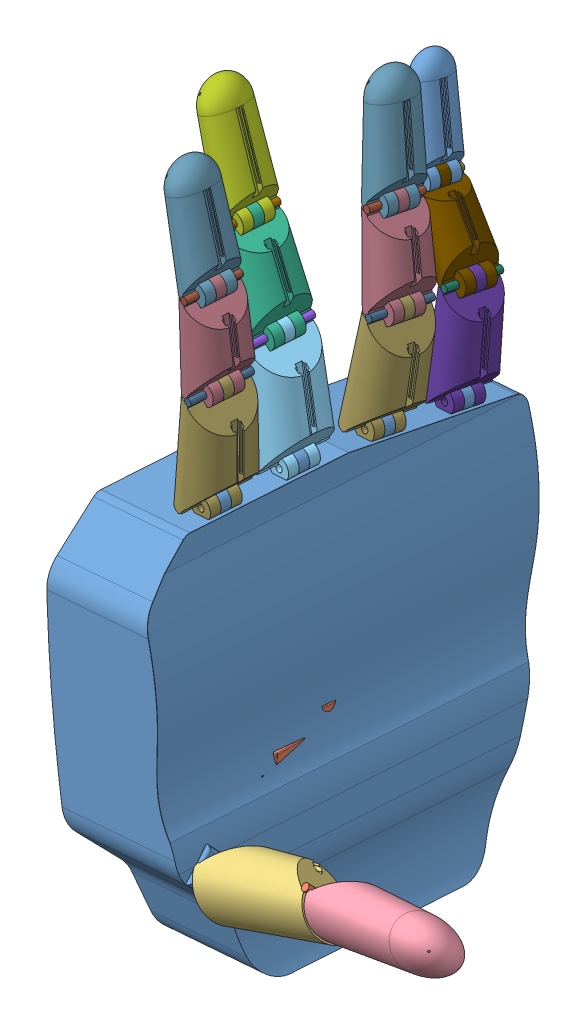
SolidWorks assembly hand_ass, configuration Default. Lengths in mm.
Overall size (398.4 729.74 146.06).
29 component instances, 20 part files, 46 mates.
Components (placement in the parent):
- mainbody_v2-4: mainbody_v2 [Default] at (1134.5845 69.0185 158.0505) x (0.046641 -0.018599 -0.998739) z (0.99192 0.118954 0.044107) size (116.82 635.31 320.58)
- Mate1t-4: Mate1t [Default] at (1191.8966 45.3831 191.6287) x (-0.116407 0.715114 0.689247) z (0.676171 0.565369 -0.472388) size (23 2 2)
- Part1t-3: Part1t [Default] at (1176.7391 49.6304 201.3469) x (-0.116407 0.715114 0.689247) z (-0.223805 0.65723 -0.719694) size (25.41 37 18.49)
- Part2t-3: Part2t [Default] at (1207.7668 55.7981 200.1909) x (-0.116407 0.715114 0.689247) z (-0.080418 0.6849 -0.724186) size (22.13 38.57 15.06)
- Part1m-2: Part1m [Default] at (1137.6384 140.5256 161.7486) x (0.046641 -0.018599 -0.998739) z (0.98582 0.162199 0.043017) size (21.28 37 15.36)
- Part2m-2: Part2m [Default] at (1130.0953 167.3581 160.8968) x (0.046641 -0.018599 -0.998739) z (0.920688 0.388657 0.035758) size (18.99 32 13.25)
- Part3m-2: Part3m [Default] at (1120.5618 193.9579 159.9559) x (0.046641 -0.018599 -0.998739) z (0.948492 0.31446 0.038438) size (16.1 35.5 11.04)
- Mate1-2: Mate1 [Default] at (1135.4417 155.2011 170.3841) x (0.046641 -0.018599 -0.998739) z (0.869405 0.4931 0.031418) size (18 2 2)
- Mate2-2: Mate2 [Default] at (1125.4133 179.1336 168.469) x (0.046641 -0.018599 -0.998739) z (0.879503 0.4748 0.032231) size (16 2 2)
- Mate1i-7: Mate1i [Default] at (1143.3187 152.4098 142.8187) x (0.061583 -0.147495 -0.987144) z (0.853826 0.519985 -0.024429) size (18 2 2)
- Mate2i-7: Mate2i [Default] at (1138.9313 172.9705 122.2515) x (-0.061583 0.147495 0.987144) z (-0.994862 0.070561 -0.072607) size (16 2 2)
- Part1i-6: Part1i [Default] at (1142.4486 137.6017 135.8591) x (0.061583 -0.147495 -0.987144) z (0.996376 -0.04906 0.069489) size (21.16 35 15.37)
- Part2-6: Part2 [Default] at (1140.4752 163.0002 131.9417) x (0.061583 -0.147495 -0.987144) z (0.972078 0.233235 0.025794) size (18.98 30 13.22)
- Part3i-6: Part3i [Default] at (1135.3592 188.4508 127.8194) x (0.061583 -0.147495 -0.987144) z (0.979901 0.196947 0.031704) size (16.1 33.51 11.04)
- Mate1p-2: Mate1p [Default] at (1142.4314 147.9759 119.6197) x (0.061583 -0.147495 -0.987144) z (0.991698 -0.102811 0.077228) size (16 2 2)
- Mate2p-2: Mate2p [Default] at (1128.4407 165.688 115.0872) x (0.061583 -0.147495 -0.987144) z (0.997523 0.042777 0.055839) size (14 2 2)
- Part1p-2: Part1p [Default] at (1142.7215 133.6027 113.6812) x (0.061583 -0.147495 -0.987144) z (0.997846 0.031496 0.057544) size (18.99 34 13.27)
- Part2p-2: Part2p [Default] at (1135.3313 155.7282 109.9141) x (0.061583 -0.147495 -0.987144) z (0.789257 0.612605 -0.042295) size (16.86 29 11.21)
- Part3p-2: Part3p [Default] at (1125.6893 177.679 106.0327) x (0.061583 -0.147495 -0.987144) z (0.9741 0.224473 0.027229) size (14.11 31.5 9.04)
- Mate1i-8: Mate1i [Default] at (1140.5368 153.6877 174.7899) x (-0.046641 0.018599 0.998739) z (-0.986648 -0.157045 -0.043151) size (18 2 2)
- Mate2i-8: Mate2i [Default] at (1137.6969 177.5363 175.215) x (-0.046641 0.018599 0.998739) z (-0.918896 -0.39289 -0.035595) size (16 2 2)
- Part1i-7: Part1i [Default] at (1139.3564 140.1863 183.9975) x (0.046641 -0.018599 -0.998739) z (0.998861 -0.009171 0.046817) size (21.16 35 15.37)
- Part2-7: Part2 [Default] at (1138.0875 166.2375 183.4538) x (0.046641 -0.018599 -0.998739) z (0.992108 0.117354 0.044146) size (18.98 30 13.22)
- Part3i-7: Part3i [Default] at (1133.0697 191.866 182.7419) x (0.046641 -0.018599 -0.998739) z (0.961902 0.270471 0.039884) size (16.1 33.51 11.04)
- SERVO 2-2: SERVO 2 [Default] at (1148.3811 12.1609 137.2372) x (0.109846 0.09566 0.989335) z (-0.993739 0.031034 0.107334) size (32 28.96 12.1)
- SERVO 2-3: SERVO 2 [Default] at (1148.2867 43.8698 121.8028) x (0.181431 0.08615 0.979623) z (-0.982404 -0.029015 0.184498) size (32 28.96 12.1)
- SERVO 2-4: SERVO 2 [Default] at (1157.2242 73.2498 119.0491) x (-0.09534 0.112725 0.989042) z (-0.991573 0.076792 -0.104336) size (32 28.96 12.1)
- SERVO 2-6: SERVO 2 [Default] at (1161.1471 38.2643 160.3978) x (0.061151 0.042032 0.997243) z (-0.997289 0.043545 0.059319) size (32 28.96 12.1)
- SERVO 2-7: SERVO 2 [Default] at (1116.2743 78.6077 176.2963) x (0.262447 -0.043955 -0.963945) z (0.96317 -0.048661 0.264455) size (32 28.96 12.1)
Mates (geometry in assembly coordinates):
- Concentric1: concentric anti-aligned: cylinder of mainbody_v2-4 through (1139.8961 124.8334 182.8072) axis (-0.046641 0.018599 0.998739) radius 1; cylinder of Part1i-7 through (1139.3299 125.0592 194.9299) axis (0.046641 -0.018599 -0.998739) radius 1
- Coincident1: coincident anti-aligned: plane of mainbody_v2-4 through (1139.8961 124.8334 182.8072) normal (0.046641 -0.018599 -0.998739); plane of Part1i-7 through (1139.8961 124.8334 182.8072) normal (-0.046641 0.018599 0.998739)
- Concentric2: concentric aligned: cylinder of Part1i-7 through (1139.6208 154.0529 194.4036) axis (0.046641 -0.018599 -0.998739) radius 1; cylinder of Part2-7 through (1139.6736 154.0319 193.2733) axis (0.046641 -0.018599 -0.998739) radius 1
- Coincident2: coincident anti-aligned: plane of Part1i-7 through (1140.047 153.883 185.277) normal (-0.046641 0.018599 0.998739); plane of Part2-7 through (1140.047 153.883 185.277) normal (0.046641 -0.018599 -0.998739)
- Concentric3: concentric aligned: cylinder of Mate1i-8 through (1139.6972 154.0225 192.7672) axis (0.046641 -0.018599 -0.998739) radius 1; cylinder of Part2-7 through (1139.6736 154.0319 193.2733) axis (0.046641 -0.018599 -0.998739) radius 1
- Coincident3: coincident anti-aligned: plane of Mate1i-8 through (1140.117 153.8551 183.7785) normal (-0.046641 0.018599 0.998739); plane of Part1i-7 through (1139.3564 140.1863 183.9975) normal (0.046641 -0.018599 -0.998739)
- Concentric4: concentric anti-aligned: cylinder of Part2-7 through (1136.8804 177.8619 192.6991) axis (0.046641 -0.018599 -0.998739) radius 1; cylinder of Part3i-7 through (1137.6736 177.5456 175.7142) axis (-0.046641 0.018599 0.998739) radius 1
- Coincident4: coincident anti-aligned: plane of Part2-7 through (1137.3937 177.6572 181.7066) normal (0.046641 -0.018599 -0.998739); plane of Part3i-7 through (1137.3937 177.6572 181.7066) normal (-0.046641 0.018599 0.998739)
- Concentric5: concentric anti-aligned: cylinder of Mate2i-8 through (1136.9506 177.8339 191.1948) axis (0.046641 -0.018599 -0.998739) radius 1; cylinder of Part3i-7 through (1137.6736 177.5456 175.7142) axis (-0.046641 0.018599 0.998739) radius 1
- Coincident5: coincident anti-aligned: plane of Mate2i-8 through (1137.3237 177.6851 183.2049) normal (-0.046641 0.018599 0.998739); plane of Part2-7 through (1138.0875 166.2375 183.4538) normal (0.046641 -0.018599 -0.998739)
- Concentric6: concentric anti-aligned: cylinder of mainbody_v2-4 through (1140.9285 124.4218 160.7001) axis (-0.046641 0.018599 0.998739) radius 1; cylinder of Part1m-2 through (1140.3622 124.6476 172.8256) axis (0.046641 -0.018599 -0.998739) radius 1
- Coincident6: coincident anti-aligned: plane of mainbody_v2-4 through (1140.9285 124.4218 160.7001) normal (0.046641 -0.018599 -0.998739); plane of Part1m-2 through (1140.9285 124.4218 160.7001) normal (-0.046641 0.018599 0.998739)
- Concentric7: concentric aligned: cylinder of Part1m-2 through (1135.3652 155.2316 172.0227) axis (0.046641 -0.018599 -0.998739) radius 1; cylinder of Part2m-2 through (1135.4179 155.2106 170.8937) axis (0.046641 -0.018599 -0.998739) radius 1
- Coincident7: coincident anti-aligned: plane of Part1m-2 through (1135.7915 155.0616 162.8935) normal (-0.046641 0.018599 0.998739); plane of Part2m-2 through (1135.7915 155.0616 162.8935) normal (0.046641 -0.018599 -0.998739)
- Concentric8: concentric anti-aligned: cylinder of Part2m-2 through (1135.4179 155.2106 170.8937) axis (0.046641 -0.018599 -0.998739) radius 1; cylinder of Mate1-2 through (1136.2812 154.8663 152.4068) axis (-0.046641 0.018599 0.998739) radius 1
- Coincident9: coincident aligned: plane of Part1m-2 through (1137.6384 140.5256 161.7486) normal (0.046641 -0.018599 -0.998739); plane of Mate1-2 through (1135.8615 155.0337 161.3954) normal (0.046641 -0.018599 -0.998739)
- Concentric9: concentric anti-aligned: cylinder of Part2m-2 through (1125.3429 179.1617 169.9772) axis (0.046641 -0.018599 -0.998739) radius 1; cylinder of Part3m-2 through (1126.1362 178.8453 152.9883) axis (-0.046641 0.018599 0.998739) radius 1
- Coincident10: coincident anti-aligned: plane of Part2m-2 through (1125.8564 178.9569 158.9807) normal (0.046641 -0.018599 -0.998739); plane of Part3m-2 through (1125.8564 178.9569 158.9807) normal (-0.046641 0.018599 0.998739)
- Concentric10: concentric aligned: cylinder of Part3m-2 through (1126.1362 178.8453 152.9883) axis (-0.046641 0.018599 0.998739) radius 1; cylinder of Mate2-2 through (1126.1595 178.836 152.4891) axis (-0.046641 0.018599 0.998739) radius 1
- Coincident11: coincident aligned: plane of Part2m-2 through (1130.0953 167.3581 160.8968) normal (0.046641 -0.018599 -0.998739); plane of Mate2-2 through (1125.7864 178.9848 160.479) normal (0.046641 -0.018599 -0.998739)
- Concentric11: concentric aligned: cylinder of mainbody_v2-4 through (1142.0789 122.6561 139.5891) axis (0.061583 -0.147495 -0.987144) radius 1; cylinder of Part1i-6 through (1141.5162 124.0039 148.6097) axis (0.061583 -0.147495 -0.987144) radius 1
- Coincident12: coincident anti-aligned: plane of mainbody_v2-4 through (1142.2637 122.2136 136.6277) normal (0.061583 -0.147495 -0.987144); plane of Part1i-6 through (1142.2637 122.2136 136.6277) normal (-0.061583 0.147495 0.987144)
- Concentric12: concentric aligned: cylinder of Part1i-6 through (1143.2179 152.6514 144.4355) axis (0.061583 -0.147495 -0.987144) radius 1; cylinder of Part2-6 through (1143.2876 152.4845 143.3183) axis (0.061583 -0.147495 -0.987144) radius 1
- Coincident13: coincident anti-aligned: plane of Part1i-6 through (1143.9654 150.8611 132.4534) normal (0.061583 -0.147495 -0.987144); plane of Part2-6 through (1143.9654 150.8611 132.4534) normal (-0.061583 0.147495 0.987144)
- Concentric13: concentric anti-aligned: cylinder of Mate1i-7 through (1144.4272 149.7549 125.0501) axis (-0.061583 0.147495 0.987144) radius 1; cylinder of Part2-6 through (1143.2876 152.4845 143.3183) axis (0.061583 -0.147495 -0.987144) radius 1
- Coincident14: coincident aligned: plane of Mate1i-7 through (1143.873 151.0824 133.9344) normal (0.061583 -0.147495 -0.987144); plane of Part2-6 through (1140.4752 163.0002 131.9417) normal (0.061583 -0.147495 -0.987144)
- Concentric14: concentric anti-aligned: cylinder of Part2-6 through (1137.8532 175.5526 139.5325) axis (0.061583 -0.147495 -0.987144) radius 1; cylinder of Part3i-6 through (1138.9005 173.0442 122.7448) axis (-0.061583 0.147495 0.987144) radius 1
- Coincident15: coincident anti-aligned: plane of Part2-6 through (1138.531 173.9292 128.6677) normal (0.061583 -0.147495 -0.987144); plane of Part3i-6 through (1138.531 173.9292 128.6677) normal (-0.061583 0.147495 0.987144)
- Concentric15: concentric anti-aligned: cylinder of Mate2i-7 through (1137.946 175.3304 138.0458) axis (0.061583 -0.147495 -0.987144) radius 1; cylinder of Part3i-6 through (1138.9005 173.0442 122.7448) axis (-0.061583 0.147495 0.987144) radius 1
- Coincident16: coincident anti-aligned: plane of Mate2i-7 through (1138.4386 174.1504 130.1486) normal (-0.061583 0.147495 0.987144); plane of Part2-6 through (1140.4752 163.0002 131.9417) normal (0.061583 -0.147495 -0.987144)
- Concentric16: concentric aligned: cylinder of mainbody_v2-4 through (1143.4645 119.3374 117.3784) axis (0.061583 -0.147495 -0.987144) radius 1; cylinder of Part1p-2 through (1142.971 120.5194 125.2891) axis (0.061583 -0.147495 -0.987144) radius 1
- Coincident17: coincident anti-aligned: plane of mainbody_v2-4 through (1143.6493 118.895 114.417) normal (0.061583 -0.147495 -0.987144); plane of Part1p-2 through (1143.6493 118.895 114.417) normal (-0.061583 0.147495 0.987144)
- Concentric17: concentric aligned: cylinder of Part1p-2 through (1142.3381 148.1991 121.1138) axis (0.061583 -0.147495 -0.987144) radius 1; cylinder of Part2p-2 through (1142.4027 148.0445 120.0789) axis (0.061583 -0.147495 -0.987144) radius 1
- Coincident18: coincident anti-aligned: plane of Part1p-2 through (1143.0164 146.5747 110.2417) normal (0.061583 -0.147495 -0.987144); plane of Part2p-2 through (1143.0164 146.5747 110.2417) normal (-0.061583 0.147495 0.987144)
- Concentric18: concentric anti-aligned: cylinder of Mate1p-2 through (1143.4167 145.616 103.8254) axis (-0.061583 0.147495 0.987144) radius 1; cylinder of Part2p-2 through (1142.4027 148.0445 120.0789) axis (0.061583 -0.147495 -0.987144) radius 1
- Coincident19: coincident aligned: plane of Mate1p-2 through (1142.924 146.7959 111.7226) normal (0.061583 -0.147495 -0.987144); plane of Part1p-2 through (1142.7215 133.6027 113.6812) normal (0.061583 -0.147495 -0.987144)
- Concentric19: concentric anti-aligned: cylinder of Part2p-2 through (1128.3505 165.9041 116.5337) axis (0.061583 -0.147495 -0.987144) radius 1; cylinder of Part3p-2 through (1129.3336 163.5493 100.7736) axis (-0.061583 0.147495 0.987144) radius 1
- Coincident20: coincident anti-aligned: plane of Part2p-2 through (1128.9642 164.4343 106.6965) normal (0.061583 -0.147495 -0.987144); plane of Part3p-2 through (1128.9642 164.4343 106.6965) normal (-0.061583 0.147495 0.987144)
- Concentric20: concentric aligned: cylinder of Mate2p-2 through (1129.3029 163.6231 101.2672) axis (-0.061583 0.147495 0.987144) radius 1; cylinder of Part3p-2 through (1129.3336 163.5493 100.7736) axis (-0.061583 0.147495 0.987144) radius 1
- Coincident21: coincident aligned: plane of Mate2p-2 through (1128.8718 164.6555 108.1772) normal (0.061583 -0.147495 -0.987144); plane of Part2p-2 through (1135.3313 155.7282 109.9141) normal (0.061583 -0.147495 -0.987144)
- Concentric21: concentric anti-aligned: cylinder of mainbody_v2-4 through (1160.386 47.3007 203.1788) axis (0.116407 -0.715114 -0.689247) radius 1; cylinder of Part1t-3 through (1162.0474 37.094 193.3413) axis (-0.116407 0.715114 0.689247) radius 1
- Coincident22: coincident anti-aligned: plane of mainbody_v2-4 through (1160.386 47.3007 203.1788) normal (-0.116407 0.715114 0.689247); plane of Part1t-3 through (1160.386 47.3007 203.1788) normal (0.116407 -0.715114 -0.689247)
- Concentric22: concentric anti-aligned: cylinder of Part1t-3 through (1192.0448 44.4731 190.7516) axis (-0.116407 0.715114 0.689247) radius 1; cylinder of Part2t-3 through (1189.6849 58.9704 204.7245) axis (0.116407 -0.715114 -0.689247) radius 1
- Coincident23: coincident anti-aligned: plane of Part1t-3 through (1190.3833 54.6797 200.589) normal (-0.116407 0.715114 0.689247); plane of Part2t-3 through (1190.3833 54.6797 200.589) normal (0.116407 -0.715114 -0.689247)
- Concentric23: concentric aligned: cylinder of Mate1t-4 through (1189.2193 61.8308 207.4814) axis (0.116407 -0.715114 -0.689247) radius 1; cylinder of Part2t-3 through (1189.6849 58.9704 204.7245) axis (0.116407 -0.715114 -0.689247) radius 1
- Coincident24: coincident aligned: plane of Mate1t-4 through (1190.558 53.6069 199.555) normal (-0.116407 0.715114 0.689247); plane of Part1t-3 through (1176.7391 49.6304 201.3469) normal (-0.116407 0.715114 0.689247)
